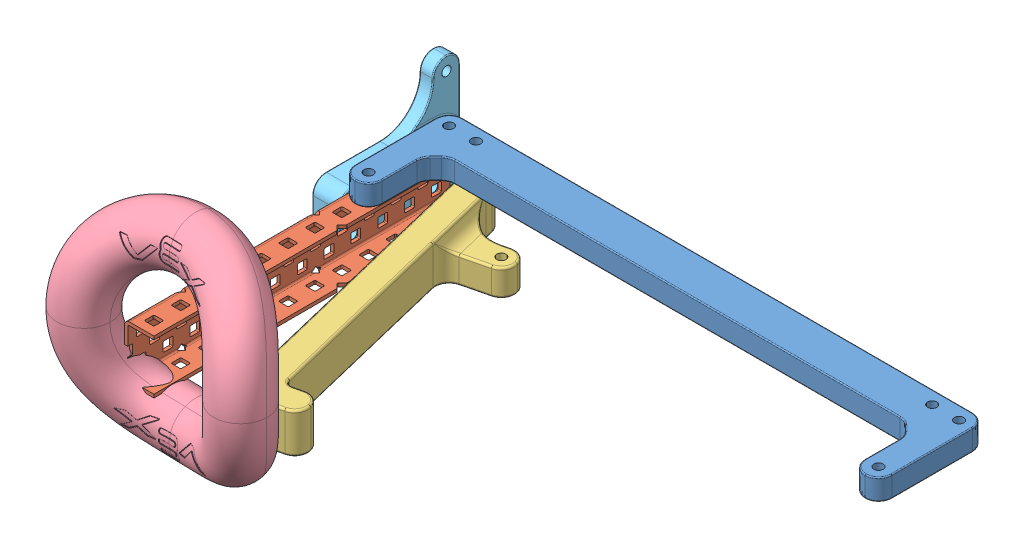
SolidWorks assembly RingMechAssem, configuration Default. Lengths in mm.
Overall size (283.05 104.58 185.15).
9 component instances, 5 part files, 9 mates.
Components (placement in the parent):
- top_brace-1: top_brace [Default] at (138.3338 128.7715 174.5683) size (254 10 50.8)
- 1x2x1x12 Aluminum C-Channel-1: 1x2x1x12 Aluminum C-Channel [Default] at (10.0638 116.0715 396.8183) x (0 0 1) z (-1 0 0) size (152.4 25.41 13.97)
- ring_hook-1: ring_hook [Default] at (22.7129 103.3715 176.2491) x (0.971667 0 -0.236353) z (0.236353 0 0.971667) size (38.1 19.4 152.4)
- Ring-1: Ring [Default] at (61.3576 128.7715 325.8457) x (0.999643 0 0.026737) z (0 1 0) size (101.61 43.55 104.58)
  - Ring.step-1: Ring.step [Default] at origin size (101.61 43.55 104.58)
    - 276-7048-350 Rev2.step-1: 276-7048-350 Rev2.step [Default] at (-27.7593 -20.073 1639.1281) size (101.61 43.55 104.58)
      - 276-7048-301 Rev2 (1).step-1: 276-7048-301 Rev2 (1).step [Default] at (0 0 -1197.0106) x (0 0 -1) z (1 0 0) size (104.58 43.55 101.61)
        - 276-7048-001 Rev2.step-1: 276-7048-001 Rev2.step [Default] at (442.1175 9.4315 0) size (104.58 43.55 101.61)
- hinge-1: hinge [Default] at (3.7138 154.1715 161.8683) x (0 0 1) z (0 -1 0) size (63.99 12.7 50.8)
Mates (geometry in assembly coordinates):
- Coincident1: coincident anti-aligned: plane of top_brace-1 through (138.3338 128.7715 174.5683) normal (0 -1 0); plane of 1x2x1x12 Aluminum C-Channel-1 through (-22.2949 128.7715 175.0683) normal (0 1 0)
- Concentric1: concentric anti-aligned: cylinder of top_brace-1 through (17.6838 138.7715 180.9183) axis (0 -1 0) radius 2.2; circle of 1x2x1x12 Aluminum C-Channel-1
- Concentric2: concentric anti-aligned: cylinder of top_brace-1 through (17.6838 138.7715 219.0183) axis (0 -1 0) radius 2.2; circle of 1x2x1x12 Aluminum C-Channel-1
- Distance1: distance = 6.35 mm anti-aligned: plane of ring_hook-1 through (22.7129 122.4215 176.2491) normal (0 1 0); plane of top_brace-1 through (138.3338 128.7715 174.5683) normal (0 -1 0)
- Concentric3: concentric aligned: cylinder of top_brace-1 through (30.3838 138.7715 180.9183) axis (0 -1 0) radius 2.2; cylinder of ring_hook-1 through (30.3838 122.4215 180.9183) axis (0 -1 0) radius 2.2
- Coincident3: coincident anti-aligned: plane of 1x2x1x12 Aluminum C-Channel-1 through (-22.2949 128.7715 175.0683) normal (0 1 0); circle of Ring-1/Ring.step-1/276-7048-350 Rev2.step-1/276-7048-301 Rev2 (1).step-1/276-7048-001 Rev2.step-1
- Coincident4: coincident anti-aligned: plane of 1x2x1x12 Aluminum C-Channel-1 through (10.0638 94.1512 175.0683) normal (-1 0 0); plane of hinge-1 through (10.0638 154.1715 161.8683) normal (1 0 0)
- Coincident5: coincident aligned: plane of 1x2x1x12 Aluminum C-Channel-1 through (-22.2949 128.7715 175.0683) normal (0 1 0); plane of hinge-1 through (-2.6362 128.7715 161.8683) normal (0 1 0)
- Distance2: distance = 12.7 mm aligned: plane of 1x2x1x12 Aluminum C-Channel-1 through (11.6386 94.1512 174.5683) normal (0 0 -1); plane of hinge-1 through (-2.6362 154.1715 161.8683) normal (0 0 -1)
